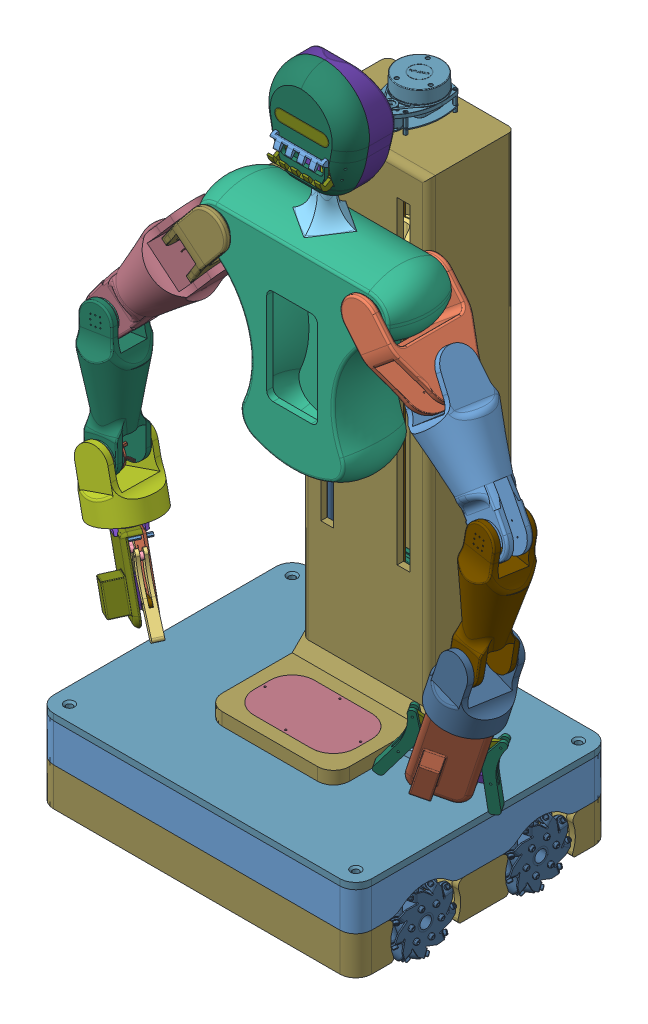
SolidWorks assembly total assembly of jaloul, configuration Défaut. Lengths in mm.
Overall size (783.33 1093.43 400).
399 component instances, 106 part files, 53 mates.
Components (placement in the parent):
- assembly bas robot jlayla-1: assembly bas robot jlayla [Défaut] at (49.7024 28.7761 8) size (508 175.73 400)
  - BASE ROBOT JALOUL-1: BASE ROBOT JALOUL [Défaut] at (-7.6983 -70.0077 500) size (500 80 400)
  - NEMA_235628-6.35_s.STEP-1: NEMA_235628-6.35_s.STEP [Défaut] at (-154.7901 -90.8073 611.8718) size (82 61.91 56.65)
    - Nema2356_top.STEP-1: Nema2356_top.STEP [Défaut] at (-25.5081 -82.6274 143.9932) size (12.4 56.42 56.42)
    - Nema2356_middle.STEP-1: Nema2356_middle.STEP [Défaut] at (-14.7081 17.769 14.044) size (32.8 56.4 56.4)
    - Nema2356_bottom.STEP-1: Nema2356_bottom.STEP [Défaut] at (18.0919 -112.7781 -165.2225) size (11 56.4 56.4)
    - Nema2356_axis.STEP-1: Nema2356_axis.STEP [Défaut] at (-52.9081 -12.2004 -20.8718) x (1 0 0) z (0 -0.367241 0.930126) size (78 6.35 6.35)
    - Nema2356_gultnis.STEP-1: Nema2356_gultnis.STEP [Défaut] at (-25.7081 -12.2004 -20.8718) x (1 0 0) z (0 0.415119 0.909767) size (3 11.6 11.6)
    - Nema2356_gultnis.STEP-2: Nema2356_gultnis.STEP [Défaut] at (22.0919 -12.2004 -20.8718) size (3 11.6 11.6)
    - Nema2356_screv.STEP-1: Nema2356_screv.STEP [Défaut] at (-13.1349 -28.2433 4.9528) size (54.01 5 5)
    - Nema2356_screv.STEP-2: Nema2356_screv.STEP [Défaut] at (-13.1349 3.8425 4.9528) size (54.01 5 5)
    - Nema2356_screv.STEP-3: Nema2356_screv.STEP [Défaut] at (-13.1349 -28.2433 -46.6964) size (54.01 5 5)
    - Nema2356_screv.STEP-4: Nema2356_screv.STEP [Défaut] at (-13.1349 3.8425 -46.6964) size (54.01 5 5)
    - Nema2356_contact.STEP-1: Nema2356_contact.STEP [Défaut] at (21.7519 15.9996 -20.8718) size (7.63 5.5 30.97)
  - support nema A 23 hee-1: support nema A 23 hee [Défaut] at (-180.2983 -103.0077 591) x (0 0 -1) z (-1 0 0) size (56 61 45)
  - Mecanum Wheel (dia 100)-1: Mecanum Wheel (dia 100) [Default] at (-192.6739 -101.7163 545.4553) x (0 -0.769085 0.639147) z (-1 0 0) size (104.21 104.22 58)
  - accouplement stpper with mecanum wheel-1: accouplement stpper with mecanum wheel [Défaut] at (-207.6983 -103.0077 591) x (0 -0.751439 0.659802) z (-1 0 0) size (18 18 35)
  - Mecanum Wheel (dia 100)-3: Mecanum Wheel (dia 100) [Default] at (177.2774 -146.933 583.0326) x (0 0.769085 -0.639147) z (1 0 0) size (104.21 104.22 58)
  - accouplement stpper with mecanum wheel-3: accouplement stpper with mecanum wheel [Défaut] at (192.3017 -103.0077 591) x (0 -0.751439 0.659802) z (1 0 0) size (18 18 35)
  - support nema A 23 hee-2: support nema A 23 hee [Défaut] at (164.9017 -103.0077 591) x (0 0 1) z (1 0 0) size (56 61 45)
  - Mecanum Wheel (dia 100)-4: Mecanum Wheel (dia 100) [Default] at (-192.6739 -146.933 416.9674) x (0 0.769085 0.639147) z (-1 0 0) size (104.21 104.22 58)
  - accouplement stpper with mecanum wheel-4: accouplement stpper with mecanum wheel [Défaut] at (-207.6983 -103.0077 409) x (0 -0.751439 -0.659802) z (-1 0 0) size (18 18 35)
  - support nema A 23 hee-3: support nema A 23 hee [Défaut] at (-180.2983 -103.0077 409) x (0 0 -1) z (-1 0 0) size (56 61 45)
  - support nema A 23 hee-4: support nema A 23 hee [Défaut] at (164.9017 -103.0077 409) x (0 0 1) z (1 0 0) size (56 61 45)
  - Mecanum Wheel (dia 100)-5: Mecanum Wheel (dia 100) [Default] at (177.2774 -102.9943 364.0959) x (0 0.769085 0.639147) z (1 0 0) size (104.21 104.22 58)
  - accouplement stpper with mecanum wheel-5: accouplement stpper with mecanum wheel [Défaut] at (192.3017 -103.0077 409) x (0 -0.751439 -0.659802) z (1 0 0) size (18 18 35)
  - NEMA_235628-6.35_s.STEP-2: NEMA_235628-6.35_s.STEP [Défaut] at (139.3936 -123.8795 578.7996) x (-1 0 0) z (0 -1 0) size (82 61.91 56.65)
    - Nema2356_top.STEP-1: Nema2356_top.STEP [Défaut] at (-25.5081 -82.6274 143.9932) size (12.4 56.42 56.42)
    - Nema2356_middle.STEP-1: Nema2356_middle.STEP [Défaut] at (-14.7081 17.769 14.044) size (32.8 56.4 56.4)
    - Nema2356_bottom.STEP-1: Nema2356_bottom.STEP [Défaut] at (18.0919 -112.7781 -165.2225) size (11 56.4 56.4)
    - Nema2356_axis.STEP-1: Nema2356_axis.STEP [Défaut] at (-52.9081 -12.2004 -20.8718) x (1 0 0) z (0 -0.367241 0.930126) size (78 6.35 6.35)
    - Nema2356_gultnis.STEP-1: Nema2356_gultnis.STEP [Défaut] at (-25.7081 -12.2004 -20.8718) x (1 0 0) z (0 0.415119 0.909767) size (3 11.6 11.6)
    - Nema2356_gultnis.STEP-2: Nema2356_gultnis.STEP [Défaut] at (22.0919 -12.2004 -20.8718) size (3 11.6 11.6)
    - Nema2356_screv.STEP-1: Nema2356_screv.STEP [Défaut] at (-13.1349 -28.2433 4.9528) size (54.01 5 5)
    - Nema2356_screv.STEP-2: Nema2356_screv.STEP [Défaut] at (-13.1349 3.8425 4.9528) size (54.01 5 5)
    - Nema2356_screv.STEP-3: Nema2356_screv.STEP [Défaut] at (-13.1349 -28.2433 -46.6964) size (54.01 5 5)
    - Nema2356_screv.STEP-4: Nema2356_screv.STEP [Défaut] at (-13.1349 3.8425 -46.6964) size (54.01 5 5)
    - Nema2356_contact.STEP-1: Nema2356_contact.STEP [Défaut] at (21.7519 15.9996 -20.8718) size (7.63 5.5 30.97)
  - NEMA_235628-6.35_s.STEP-3: NEMA_235628-6.35_s.STEP [Défaut] at (139.3936 -90.8073 388.1282) x (-1 0 0) z (0 0 -1) size (82 61.91 56.65)
    - Nema2356_top.STEP-1: Nema2356_top.STEP [Défaut] at (-25.5081 -82.6274 143.9932) size (12.4 56.42 56.42)
    - Nema2356_middle.STEP-1: Nema2356_middle.STEP [Défaut] at (-14.7081 17.769 14.044) size (32.8 56.4 56.4)
    - Nema2356_bottom.STEP-1: Nema2356_bottom.STEP [Défaut] at (18.0919 -112.7781 -165.2225) size (11 56.4 56.4)
    - Nema2356_axis.STEP-1: Nema2356_axis.STEP [Défaut] at (-52.9081 -12.2004 -20.8718) x (1 0 0) z (0 -0.367241 0.930126) size (78 6.35 6.35)
    - Nema2356_gultnis.STEP-1: Nema2356_gultnis.STEP [Défaut] at (-25.7081 -12.2004 -20.8718) x (1 0 0) z (0 0.415119 0.909767) size (3 11.6 11.6)
    - Nema2356_gultnis.STEP-2: Nema2356_gultnis.STEP [Défaut] at (22.0919 -12.2004 -20.8718) size (3 11.6 11.6)
    - Nema2356_screv.STEP-1: Nema2356_screv.STEP [Défaut] at (-13.1349 -28.2433 4.9528) size (54.01 5 5)
    - Nema2356_screv.STEP-2: Nema2356_screv.STEP [Défaut] at (-13.1349 3.8425 4.9528) size (54.01 5 5)
    - Nema2356_screv.STEP-3: Nema2356_screv.STEP [Défaut] at (-13.1349 -28.2433 -46.6964) size (54.01 5 5)
    - Nema2356_screv.STEP-4: Nema2356_screv.STEP [Défaut] at (-13.1349 3.8425 -46.6964) size (54.01 5 5)
    - Nema2356_contact.STEP-1: Nema2356_contact.STEP [Défaut] at (21.7519 15.9996 -20.8718) size (7.63 5.5 30.97)
  - NEMA_235628-6.35_s.STEP-4: NEMA_235628-6.35_s.STEP [Défaut] at (-154.7901 -90.8073 429.8718) size (82 61.91 56.65)
    - Nema2356_top.STEP-1: Nema2356_top.STEP [Défaut] at (-25.5081 -82.6274 143.9932) size (12.4 56.42 56.42)
    - Nema2356_middle.STEP-1: Nema2356_middle.STEP [Défaut] at (-14.7081 17.769 14.044) size (32.8 56.4 56.4)
    - Nema2356_bottom.STEP-1: Nema2356_bottom.STEP [Défaut] at (18.0919 -112.7781 -165.2225) size (11 56.4 56.4)
    - Nema2356_axis.STEP-1: Nema2356_axis.STEP [Défaut] at (-52.9081 -12.2004 -20.8718) x (1 0 0) z (0 -0.367241 0.930126) size (78 6.35 6.35)
    - Nema2356_gultnis.STEP-1: Nema2356_gultnis.STEP [Défaut] at (-25.7081 -12.2004 -20.8718) x (1 0 0) z (0 0.415119 0.909767) size (3 11.6 11.6)
    - Nema2356_gultnis.STEP-2: Nema2356_gultnis.STEP [Défaut] at (22.0919 -12.2004 -20.8718) size (3 11.6 11.6)
    - Nema2356_screv.STEP-1: Nema2356_screv.STEP [Défaut] at (-13.1349 -28.2433 4.9528) size (54.01 5 5)
    - Nema2356_screv.STEP-2: Nema2356_screv.STEP [Défaut] at (-13.1349 3.8425 4.9528) size (54.01 5 5)
    - Nema2356_screv.STEP-3: Nema2356_screv.STEP [Défaut] at (-13.1349 -28.2433 -46.6964) size (54.01 5 5)
    - Nema2356_screv.STEP-4: Nema2356_screv.STEP [Défaut] at (-13.1349 3.8425 -46.6964) size (54.01 5 5)
    - Nema2356_contact.STEP-1: Nema2356_contact.STEP [Défaut] at (21.7519 15.9996 -20.8718) size (7.63 5.5 30.97)
  - cache base joulayla-1: cache base joulayla [Défaut] at (-6.3132 -120.0077 499.8615) x (1 0 0) z (0 1 0) size (500 400 60)
  - profilé support base jlayla-1: profilé support base jlayla [Varsayılan] at (217.3017 -60.0077 675) x (1 0 0) z (0 1 0) size (25 25 50)
  - profilé support base jlayla-2: profilé support base jlayla [Varsayılan] at (-232.6983 -10.0077 675) x (-1 0 0) z (0 -1 0) size (25 25 50)
  - profilé support base jlayla-3: profilé support base jlayla [Varsayılan] at (217.3017 -10.0077 325) x (1 0 0) z (0 -1 0) size (25 25 50)
  - profilé support base jlayla-4: profilé support base jlayla [Varsayılan] at (-232.6983 -60.0077 325) x (-1 0 0) z (0 1 0) size (25 25 50)
  - profilé support base jlayla-5: profilé support base jlayla [Varsayılan] at (-7.6983 -60.0077 500) x (-1 0 0) z (0 1 0) size (25 25 50)
  - cache supérieur fixe jlayla-1: cache supérieur fixe jlayla [Défaut] at (-7.4213 -10.0077 499.0305) x (-1 0 0) z (0 1 0) size (500 400 10)
- assemblt jaloul main two-1: assemblt jaloul main two [Défaut] at (-8.2808 774.6085 403.5033) x (0.999385 -0.035073 0) z (0 0 1) size (752.19 900.92 286)
  - assembly head of jaloul-1: assembly head of jaloul [Défaut] at (50.4629 78.1935 73.0866) x (0.999385 0.035073 0) z (0 0 1) size (153.86 218.57 97.38)
    - head of jaloul-1: head of jaloul [Défaut] at (-2.8889 8.1989 56.9742) size (153.86 167.94 40.08)
    - RealSense_D435-1: RealSense_D435 [Default] at (-2 5.7058 43.2445) size (90.75 24.75 24.23)
    - ras jaloul men teli-1: ras jaloul men teli [Défaut] at (-4.3071 -4.0651 25.143) size (140.75 169.26 46.26)
    - raspberry-pi-5-sbc-simple.step-1: raspberry-pi-5-sbc-simple.step [Défaut] at (-2.8895 30.0633 18.143) size (90.56 58 19.2)
      - CSI_DSI-1.step-1: CSI_DSI-1.step [Défaut] at (-70.5 -36 11.75) size (3 15.5 4.1)
        - CSI_DSI_connector.step-1: CSI_DSI_connector.step [Défaut] at origin size (3 15.5 4.1)
      - CSI_DSI-2.step-1: CSI_DSI-2.step [Défaut] at (-70.5 -36 11.75) size (3 15.5 4.1)
        - CSI_DSI_connector.step-1: CSI_DSI_connector.step [Défaut] at (6.2 0 0) size (3 15.5 4.1)
      - pcba-components.step-1: pcba-components.step [Défaut] at (-70.5 -36 11.75) size (64.89 40.96 3.37)
        - pcba-components Geometry.step-1: pcba-components Geometry.step [Défaut] at origin size (62.02 39.27 3.37)
        - chips.step-1: chips.step [Défaut] at origin size (13.6 15 1)
      - poe.step-1: poe.step [Défaut] at (-70.5 -36 11.75) size (5.08 5.08 8.29)
        - poe Geometry.step-1: poe Geometry.step [Défaut] at origin size (5.08 5.08 1)
        - poe-pins.step-1: poe-pins.step [Défaut] at origin size (3.44 3.44 7.29)
      - usb-2-bank.step-1: usb-2-bank.step [Défaut] at (-0.7443 20 0.8) x (1 0 0) z (0 -1 0) size (17.07 15.5 13.76)
        - usb-2-bank Geometry.step-1: usb-2-bank Geometry.step [Défaut] at origin size (16.67 15.5 13.76)
        - usb2-port.step-1: usb2-port.step [Défaut] at origin size (4.42 5.12 12.5)
        - usb2-port.step-2: usb2-port.step [Défaut] at (0 -8.5 0) size (4.42 5.12 12.5)
      - usb-3-bank.step-1: usb-3-bank.step [Défaut] at (-0.5443 2.1 0.8) x (1 0 0) z (0 -1 0) size (17.07 15.5 13.76)
        - usb-3-bank Geometry.step-1: usb-3-bank Geometry.step [Défaut] at origin size (16.67 15.5 13.76)
        - usb3-port.step-1: usb3-port.step [Défaut] at origin size (4.42 5.12 12.5)
        - usb3-port.step-2: usb3-port.step [Défaut] at (0 -8.5 0) size (4.42 5.12 12.5)
      - connector.step-1: connector.step [Défaut] at (-70.5 -36 11.75) size (3 6 3.5)
      - ethernet.step-1: ethernet.step [Défaut] at (0 -35.55 0.8) x (1 0 0) z (0 -1 0) size (23.65 17.25 16)
      - gpio.step-1: gpio.step [Défaut] at (-70.53 -36.28 11.75) size (50.5 5 8.29)
      - hdmi-micro.step-1: hdmi-micro.step [Défaut] at (-0.3 0 0.8) x (1 0 0) z (0 -1 0) size (6.5 2.9 7.7)
      - hdmi-micro.step-2: hdmi-micro.step [Défaut] at (-13.8 0 0.8) x (1 0 0) z (0 -1 0) size (6.5 2.9 7.7)
      - IR.step-1: IR.step [Défaut] at (-70.5 -36 11.75) size (1.73 3.15 3.26)
      - mounting-holes.step-1: mounting-holes.step [Défaut] at (-70.5 -36 11.75) size (64 54.91 0.02)
      - pcb.step-1: pcb.step [Défaut] at (-70.5 -36 11.75) size (85 56 1.6)
      - pcie.step-1: pcie.step [Défaut] at (-70.5 -36 11.75) size (3 10.5 4.1)
      - pmic.step-1: pmic.step [Défaut] at (-70.5 -36 11.75) size (6 6 0.5)
      - pwr-connector.step-1: pwr-connector.step [Défaut] at (-70.5 -36 11.75) size (4 3 4.4)
      - rp1.step-1: rp1.step [Défaut] at (-70.5 -36 11.75) size (12 12 0.5)
      - sd-card.step-1: sd-card.step [Défaut] at (-70.5 -36 11.75) size (1.75 11.01 0.01) (hidden)
      - switch.step-1: switch.step [Défaut] at (-70.5 -36 11.75) size (3 4.75 1.77)
      - uart.step-1: uart.step [Défaut] at (-70.5 -36 11.75) size (5.25 3.25 4.4)
      - usb-c.step-1: usb-c.step [Défaut] at (-70.5 -36 11.75) size (9 7.5 3.2)
    - support head-1: support head [Défaut] at (-2.8895 -82.9367 30.143) x (0.544466 0 -0.838783) z (0 -1 0) size (62.95 62.95 55.38)
    - M90S_ali.step-1: M90S_ali.step [Défaut] at (23.3 -47.0367 54.243) x (0 -1 0) z (1 0 0) size (32.3 12.4 32.5)
      - axe.step-1: axe.step [Défaut] at origin size (4.9 4.9 14.2)
      - base001.step-1: base001.step [Défaut] at origin size (32.3 12.2 28.5)
      - etiquette.step-1: etiquette.step [Défaut] at origin size (20 0.2 10)
      - Tube.step-1: Tube.step [Défaut] at (5.4 0 -13.3) x (0 0 -1) z (1 0 0) size (1.2 1.2 3)
      - Cylindre.step-1: Cylindre.step [Défaut] at (5.4 0 -13.3) x (0 0 -1) z (1 0 0) size (0.4 0.4 4)
      - Tube001.step-1: Tube001.step [Défaut] at (5.4 -1.2 -13.3) x (0 0 -1) z (1 0 0) size (1.2 1.2 3)
      - Tube002.step-1: Tube002.step [Défaut] at (5.4 1.2 -13.3) x (0 0 -1) z (1 0 0) size (1.2 1.2 3)
      - etiquette001.step-1: etiquette001.step [Défaut] at (-10.8 0 0) x (-1 0 0) z (0 0 1) size (20 0.2 10)
      - Cylindre001.step-1: Cylindre001.step [Défaut] at (5.4 1.2 -13.3) x (0 0 -1) z (1 0 0) size (0.4 0.4 4)
      - Cylindre002.step-1: Cylindre002.step [Défaut] at (5.4 -1.2 -13.3) x (0 0 -1) z (1 0 0) size (0.4 0.4 4)
    - dents du jaloul-1: dents du jaloul [Défaut] at (-1.85 -55.3304 58.7391) x (-1 0 0) z (0 0.870081 0.492909) size (83 33.18 25.45)
    - MG90S_arm01.step-1: MG90S_arm01.step [Défaut] at (39.3 -47.0367 54.243) x (-1 0 0) z (0 0.870081 0.492909) size (4.8 21.4 6.8)
    - dent jaloul partie supérieur-1: dent jaloul partie supérieur [Défaut] at (-1.85 5.574 3.1017) size (83 33.18 25.45)
    - Symétriedents du jaloul-4: Symétriedents du jaloul [Défaut] at (-1.85 -21.043 58.7391) x (-1 0 0) z (0 0.870081 -0.492909) size (83 32.99 25.26)
  - 4015 Motor.STEP-1: 4015 Motor.STEP [Défaut] at (-65.9697 -107.9474 135.4967) x (-0.675127 -0.737702 0) z (-0.737702 0.675127 0) size (63.54 36.6 63.54)
    - 4015定子.STEP-1: 4015定子.STEP [Défaut] at origin size (45.94 27.09 45.92)
    - MISUMI_C-E6800ZZ.STEP-1: MISUMI_C-E6800ZZ.STEP [Défaut] at (0 21.6 0) x (0 -1 0) z (-0.009932 0 0.999951) size (5 19 19)
    - MISUMI_C-E6800ZZ.STEP-2: MISUMI_C-E6800ZZ.STEP [Défaut] at (0 8 0) x (0 -1 0) z (-0.587995 0 0.808864) size (5 19 19)
    - 转子铝盖.STEP-1: 转子铝盖.STEP [Défaut] at (0 24 0) x (-0.665718 0 -0.746203) z (-0.746203 0 0.665718) size (45 23.5 45)
    - 磁钢片.STEP-1: 磁钢片.STEP [Défaut] at (5.7872 12.75 -20.8182) x (0.963466 0 0.267832) z (-0.267832 0 0.963466) size (4 16.5 1.3)
    - 中间不锈钢圈.STEP-1: 中间不锈钢圈.STEP [Défaut] at (0 4.5 0) x (0.999998 0 0.002002) z (0 1 0) size (45 45 16.5)
    - 磁钢片.STEP-2: 磁钢片.STEP [Défaut] at (-0.3124 12.75 -21.6054) x (0.999895 0 -0.014457) z (0.014457 0 0.999895) size (4 16.5 1.3)
    - 磁钢片.STEP-3: 磁钢片.STEP [Défaut] at (-6.3867 12.75 -20.6422) x (0.95532 0 -0.295574) z (0.295574 0 0.95532) size (4 16.5 1.3)
    - 磁钢片.STEP-4: 磁钢片.STEP [Défaut] at (-11.9435 12.75 -18.0067) x (0.83335 0 -0.552746) z (0.552746 0 0.83335) size (4 16.5 1.3)
    - 磁钢片.STEP-5: 磁钢片.STEP [Défaut] at (-16.5328 12.75 -13.9124) x (0.643867 0 -0.765138) z (0.765138 0 0.643867) size (4 16.5 1.3)
    - 磁钢片.STEP-6: 磁钢片.STEP [Défaut] at (-19.7827 12.75 -8.6911) x (0.402221 0 -0.915542) z (0.915542 0 0.402221) size (4 16.5 1.3)
    - 磁钢片.STEP-7: 磁钢片.STEP [Défaut] at (-21.4299 12.75 -2.7656) x (0.12799 0 -0.991775) z (0.991775 0 0.12799) size (4 16.5 1.3)
    - 磁钢片.STEP-8: 磁钢片.STEP [Défaut] at (-21.341 12.75 3.384) x (-0.15661 0 -0.987661) z (0.987661 0 -0.15661) size (4 16.5 1.3)
    - 磁钢片.STEP-9: 磁钢片.STEP [Défaut] at (-19.5232 12.75 9.2593) x (-0.428522 0 -0.903531) z (0.903531 0 -0.428522) size (4 16.5 1.3)
    - 磁钢片.STEP-10: 磁钢片.STEP [Défaut] at (-16.1237 12.75 14.3846) x (-0.665718 0 -0.746203) z (0.746203 0 -0.665718) size (4 16.5 1.3)
    - 磁钢片.STEP-11: 磁钢片.STEP [Défaut] at (-11.418 12.75 18.3445) x (-0.848982 0 -0.528423) z (0.528423 0 -0.848982) size (4 16.5 1.3)
    - 磁钢片.STEP-12: 磁钢片.STEP [Défaut] at (-5.7872 12.75 20.8182) x (-0.963466 0 -0.267832) z (0.267832 0 -0.963466) size (4 16.5 1.3)
    - 磁钢片.STEP-13: 磁钢片.STEP [Défaut] at (0.3124 12.75 21.6054) x (-0.999895 0 0.014457) z (-0.014457 0 -0.999895) size (4 16.5 1.3)
    - 磁钢片.STEP-14: 磁钢片.STEP [Défaut] at (6.3867 12.75 20.6422) x (-0.95532 0 0.295574) z (-0.295574 0 -0.95532) size (4 16.5 1.3)
    - 磁钢片.STEP-15: 磁钢片.STEP [Défaut] at (11.9435 12.75 18.0067) x (-0.83335 0 0.552746) z (-0.552746 0 -0.83335) size (4 16.5 1.3)
    - 磁钢片.STEP-16: 磁钢片.STEP [Défaut] at (16.5328 12.75 13.9124) x (-0.643867 0 0.765138) z (-0.765138 0 -0.643867) size (4 16.5 1.3)
    - 磁钢片.STEP-17: 磁钢片.STEP [Défaut] at (19.7827 12.75 8.6911) x (-0.402221 0 0.915542) z (-0.915542 0 -0.402221) size (4 16.5 1.3)
    - 磁钢片.STEP-18: 磁钢片.STEP [Défaut] at (21.4299 12.75 2.7656) x (-0.12799 0 0.991775) z (-0.991775 0 -0.12799) size (4 16.5 1.3)
    - 磁钢片.STEP-19: 磁钢片.STEP [Défaut] at (21.341 12.75 -3.384) x (0.15661 0 0.987661) z (-0.987661 0 0.15661) size (4 16.5 1.3)
    - 磁钢片.STEP-20: 磁钢片.STEP [Défaut] at (19.5232 12.75 -9.2593) x (0.428522 0 0.903531) z (-0.903531 0 0.428522) size (4 16.5 1.3)
    - 磁钢片.STEP-21: 磁钢片.STEP [Défaut] at (16.1237 12.75 -14.3846) x (0.665718 0 0.746203) z (-0.746203 0 0.665718) size (4 16.5 1.3)
    - 磁钢片.STEP-22: 磁钢片.STEP [Défaut] at (11.418 12.75 -18.3445) x (0.848982 0 0.528423) z (-0.528423 0 0.848982) size (4 16.5 1.3)
    - 径向磁环.STEP-1: 径向磁环.STEP [Défaut] at (0 0.5 0) x (0.972164 0 0.234302) z (0 -1 0) size (10 10 2.5)
    - 径向磁环固定环.STEP-1: 径向磁环固定环.STEP [Défaut] at (0 -2 0) x (0.933781 0 0.357846) z (0 1 0) size (11.2 12.93 5)
    - 铜柱M2.5x4+4.STEP-1: 铜柱M2.5x4+4.STEP [Défaut] at (14 -4 0) size (5 8 5.77)
    - 铜柱M2.5x4+4.STEP-2: 铜柱M2.5x4+4.STEP [Défaut] at (0 -4 -14) x (0.982082 0 -0.188455) z (0.188455 0 0.982082) size (5 8 5.77)
    - 铜柱M2.5x4+4.STEP-3: 铜柱M2.5x4+4.STEP [Défaut] at (0 -4 14) x (0.918365 0 -0.395734) z (0.395734 0 0.918365) size (5 8 5.77)
    - 铜柱M2.5x4+4.STEP-4: 铜柱M2.5x4+4.STEP [Défaut] at (-14 -4 0) x (0.8 0 -0.6) z (0.6 0 0.8) size (5 8 5.77)
    - AS5600磁编码器-圆.STEP-1: AS5600磁编码器-圆.STEP [Défaut] at (-0.3592 -5.6 0) x (0.707107 0 -0.707107) z (0 1 0) size (31.97 31.97 7.67)
    - 铜柱M2.5x7+4.STEP-1: 铜柱M2.5x7+4.STEP [Défaut] at (0 -12.6 -14) x (0.898383 0 -0.439214) z (0.439214 0 0.898383) size (5 11 5.77)
    - 铜柱M2.5x7+4.STEP-2: 铜柱M2.5x7+4.STEP [Défaut] at (-14 -12.6 0) x (0.799513 0 -0.600648) z (0.600648 0 0.799513) size (5 11 5.77)
    - 铜柱M2.5x7+4.STEP-3: 铜柱M2.5x7+4.STEP [Défaut] at (14 -12.6 0) x (0.651231 0 -0.758879) z (0.758879 0 0.651231) size (5 11 5.77)
    - 铜柱M2.5x7+4.STEP-4: 铜柱M2.5x7+4.STEP [Défaut] at (0 -12.6 14) x (0.455178 0 -0.890401) z (0.890401 0 0.455178) size (5 11 5.77)
  - link 1 JALOUL-1: link 1 JALOUL [Défaut] at (-74.3576 -118.8426 159.4967) x (0.61003 0.792378 0) z (0 0 1) size (167.5 60.6 125)
  - 4015 Motor.STEP-2: 4015 Motor.STEP [Défaut] at (-134.1638 -178.494 106.9967) x (0.604333 0.784978 0.136349) z (-0.083177 -0.10804 0.990661) size (63.54 36.6 63.54)
    - 4015定子.STEP-1: 4015定子.STEP [Défaut] at origin size (45.94 27.09 45.92)
    - MISUMI_C-E6800ZZ.STEP-1: MISUMI_C-E6800ZZ.STEP [Défaut] at (0 21.6 0) x (0 -1 0) z (-0.009932 0 0.999951) size (5 19 19)
    - MISUMI_C-E6800ZZ.STEP-2: MISUMI_C-E6800ZZ.STEP [Défaut] at (0 8 0) x (0 -1 0) z (-0.587995 0 0.808864) size (5 19 19)
    - 转子铝盖.STEP-1: 转子铝盖.STEP [Défaut] at (0 24 0) x (-0.665718 0 -0.746203) z (-0.746203 0 0.665718) size (45 23.5 45)
    - 磁钢片.STEP-1: 磁钢片.STEP [Défaut] at (5.7872 12.75 -20.8182) x (0.963466 0 0.267832) z (-0.267832 0 0.963466) size (4 16.5 1.3)
    - 中间不锈钢圈.STEP-1: 中间不锈钢圈.STEP [Défaut] at (0 4.5 0) x (0.999998 0 0.002002) z (0 1 0) size (45 45 16.5)
    - 磁钢片.STEP-2: 磁钢片.STEP [Défaut] at (-0.3124 12.75 -21.6054) x (0.999895 0 -0.014457) z (0.014457 0 0.999895) size (4 16.5 1.3)
    - 磁钢片.STEP-3: 磁钢片.STEP [Défaut] at (-6.3867 12.75 -20.6422) x (0.95532 0 -0.295574) z (0.295574 0 0.95532) size (4 16.5 1.3)
    - 磁钢片.STEP-4: 磁钢片.STEP [Défaut] at (-11.9435 12.75 -18.0067) x (0.83335 0 -0.552746) z (0.552746 0 0.83335) size (4 16.5 1.3)
    - 磁钢片.STEP-5: 磁钢片.STEP [Défaut] at (-16.5328 12.75 -13.9124) x (0.643867 0 -0.765138) z (0.765138 0 0.643867) size (4 16.5 1.3)
    - 磁钢片.STEP-6: 磁钢片.STEP [Défaut] at (-19.7827 12.75 -8.6911) x (0.402221 0 -0.915542) z (0.915542 0 0.402221) size (4 16.5 1.3)
    - 磁钢片.STEP-7: 磁钢片.STEP [Défaut] at (-21.4299 12.75 -2.7656) x (0.12799 0 -0.991775) z (0.991775 0 0.12799) size (4 16.5 1.3)
    - 磁钢片.STEP-8: 磁钢片.STEP [Défaut] at (-21.341 12.75 3.384) x (-0.15661 0 -0.987661) z (0.987661 0 -0.15661) size (4 16.5 1.3)
    - 磁钢片.STEP-9: 磁钢片.STEP [Défaut] at (-19.5232 12.75 9.2593) x (-0.428522 0 -0.903531) z (0.903531 0 -0.428522) size (4 16.5 1.3)
    - 磁钢片.STEP-10: 磁钢片.STEP [Défaut] at (-16.1237 12.75 14.3846) x (-0.665718 0 -0.746203) z (0.746203 0 -0.665718) size (4 16.5 1.3)
    - 磁钢片.STEP-11: 磁钢片.STEP [Défaut] at (-11.418 12.75 18.3445) x (-0.848982 0 -0.528423) z (0.528423 0 -0.848982) size (4 16.5 1.3)
    - 磁钢片.STEP-12: 磁钢片.STEP [Défaut] at (-5.7872 12.75 20.8182) x (-0.963466 0 -0.267832) z (0.267832 0 -0.963466) size (4 16.5 1.3)
    - 磁钢片.STEP-13: 磁钢片.STEP [Défaut] at (0.3124 12.75 21.6054) x (-0.999895 0 0.014457) z (-0.014457 0 -0.999895) size (4 16.5 1.3)
    - 磁钢片.STEP-14: 磁钢片.STEP [Défaut] at (6.3867 12.75 20.6422) x (-0.95532 0 0.295574) z (-0.295574 0 -0.95532) size (4 16.5 1.3)
    - 磁钢片.STEP-15: 磁钢片.STEP [Défaut] at (11.9435 12.75 18.0067) x (-0.83335 0 0.552746) z (-0.552746 0 -0.83335) size (4 16.5 1.3)
    - 磁钢片.STEP-16: 磁钢片.STEP [Défaut] at (16.5328 12.75 13.9124) x (-0.643867 0 0.765138) z (-0.765138 0 -0.643867) size (4 16.5 1.3)
    - 磁钢片.STEP-17: 磁钢片.STEP [Défaut] at (19.7827 12.75 8.6911) x (-0.402221 0 0.915542) z (-0.915542 0 -0.402221) size (4 16.5 1.3)
    - 磁钢片.STEP-18: 磁钢片.STEP [Défaut] at (21.4299 12.75 2.7656) x (-0.12799 0 0.991775) z (-0.991775 0 -0.12799) size (4 16.5 1.3)
    - 磁钢片.STEP-19: 磁钢片.STEP [Défaut] at (21.341 12.75 -3.384) x (0.15661 0 0.987661) z (-0.987661 0 0.15661) size (4 16.5 1.3)
    - 磁钢片.STEP-20: 磁钢片.STEP [Défaut] at (19.5232 12.75 -9.2593) x (0.428522 0 0.903531) z (-0.903531 0 0.428522) size (4 16.5 1.3)
    - 磁钢片.STEP-21: 磁钢片.STEP [Défaut] at (16.1237 12.75 -14.3846) x (0.665718 0 0.746203) z (-0.746203 0 0.665718) size (4 16.5 1.3)
    - 磁钢片.STEP-22: 磁钢片.STEP [Défaut] at (11.418 12.75 -18.3445) x (0.848982 0 0.528423) z (-0.528423 0 0.848982) size (4 16.5 1.3)
    - 径向磁环.STEP-1: 径向磁环.STEP [Défaut] at (0 0.5 0) x (0.972164 0 0.234302) z (0 -1 0) size (10 10 2.5)
    - 径向磁环固定环.STEP-1: 径向磁环固定环.STEP [Défaut] at (0 -2 0) x (0.933781 0 0.357846) z (0 1 0) size (11.2 12.93 5)
    - 铜柱M2.5x4+4.STEP-1: 铜柱M2.5x4+4.STEP [Défaut] at (14 -4 0) size (5 8 5.77)
    - 铜柱M2.5x4+4.STEP-2: 铜柱M2.5x4+4.STEP [Défaut] at (0 -4 -14) x (0.982082 0 -0.188455) z (0.188455 0 0.982082) size (5 8 5.77)
    - 铜柱M2.5x4+4.STEP-3: 铜柱M2.5x4+4.STEP [Défaut] at (0 -4 14) x (0.918365 0 -0.395734) z (0.395734 0 0.918365) size (5 8 5.77)
    - 铜柱M2.5x4+4.STEP-4: 铜柱M2.5x4+4.STEP [Défaut] at (-14 -4 0) x (0.8 0 -0.6) z (0.6 0 0.8) size (5 8 5.77)
    - AS5600磁编码器-圆.STEP-1: AS5600磁编码器-圆.STEP [Défaut] at (-0.3592 -5.6 0) x (0.707107 0 -0.707107) z (0 1 0) size (31.97 31.97 7.67)
    - 铜柱M2.5x7+4.STEP-1: 铜柱M2.5x7+4.STEP [Défaut] at (0 -12.6 -14) x (0.898383 0 -0.439214) z (0.439214 0 0.898383) size (5 11 5.77)
    - 铜柱M2.5x7+4.STEP-2: 铜柱M2.5x7+4.STEP [Défaut] at (-14 -12.6 0) x (0.799513 0 -0.600648) z (0.600648 0 0.799513) size (5 11 5.77)
    - 铜柱M2.5x7+4.STEP-3: 铜柱M2.5x7+4.STEP [Défaut] at (14 -12.6 0) x (0.651231 0 -0.758879) z (0.758879 0 0.651231) size (5 11 5.77)
    - 铜柱M2.5x7+4.STEP-4: 铜柱M2.5x7+4.STEP [Défaut] at (0 -12.6 14) x (0.455178 0 -0.890401) z (0.890401 0 0.455178) size (5 11 5.77)
  - link 2 JALOUL-1: link 2 JALOUL [Défaut] at (-194.9505 -201.7159 82.9556) x (0.606326 0.787567 -0.110033) z (0.067124 0.087188 0.993928) size (247.23 121.75 118.52)
  - 4015 Motor.STEP-3: 4015 Motor.STEP [Défaut] at (-242.3982 -333.0153 128.8669) x (-0.985892 -0.147294 0.079502) z (-0.153331 0.985242 -0.076071) size (63.54 36.6 63.54)
    - 4015定子.STEP-1: 4015定子.STEP [Défaut] at origin size (45.94 27.09 45.92)
    - MISUMI_C-E6800ZZ.STEP-1: MISUMI_C-E6800ZZ.STEP [Défaut] at (0 21.6 0) x (0 -1 0) z (-0.009932 0 0.999951) size (5 19 19)
    - MISUMI_C-E6800ZZ.STEP-2: MISUMI_C-E6800ZZ.STEP [Défaut] at (0 8 0) x (0 -1 0) z (-0.587995 0 0.808864) size (5 19 19)
    - 转子铝盖.STEP-1: 转子铝盖.STEP [Défaut] at (0 24 0) x (-0.665718 0 -0.746203) z (-0.746203 0 0.665718) size (45 23.5 45)
    - 磁钢片.STEP-1: 磁钢片.STEP [Défaut] at (5.7872 12.75 -20.8182) x (0.963466 0 0.267832) z (-0.267832 0 0.963466) size (4 16.5 1.3)
    - 中间不锈钢圈.STEP-1: 中间不锈钢圈.STEP [Défaut] at (0 4.5 0) x (0.999998 0 0.002002) z (0 1 0) size (45 45 16.5)
    - 磁钢片.STEP-2: 磁钢片.STEP [Défaut] at (-0.3124 12.75 -21.6054) x (0.999895 0 -0.014457) z (0.014457 0 0.999895) size (4 16.5 1.3)
    - 磁钢片.STEP-3: 磁钢片.STEP [Défaut] at (-6.3867 12.75 -20.6422) x (0.95532 0 -0.295574) z (0.295574 0 0.95532) size (4 16.5 1.3)
    - 磁钢片.STEP-4: 磁钢片.STEP [Défaut] at (-11.9435 12.75 -18.0067) x (0.83335 0 -0.552746) z (0.552746 0 0.83335) size (4 16.5 1.3)
    - 磁钢片.STEP-5: 磁钢片.STEP [Défaut] at (-16.5328 12.75 -13.9124) x (0.643867 0 -0.765138) z (0.765138 0 0.643867) size (4 16.5 1.3)
    - 磁钢片.STEP-6: 磁钢片.STEP [Défaut] at (-19.7827 12.75 -8.6911) x (0.402221 0 -0.915542) z (0.915542 0 0.402221) size (4 16.5 1.3)
    - 磁钢片.STEP-7: 磁钢片.STEP [Défaut] at (-21.4299 12.75 -2.7656) x (0.12799 0 -0.991775) z (0.991775 0 0.12799) size (4 16.5 1.3)
    - 磁钢片.STEP-8: 磁钢片.STEP [Défaut] at (-21.341 12.75 3.384) x (-0.15661 0 -0.987661) z (0.987661 0 -0.15661) size (4 16.5 1.3)
    - 磁钢片.STEP-9: 磁钢片.STEP [Défaut] at (-19.5232 12.75 9.2593) x (-0.428522 0 -0.903531) z (0.903531 0 -0.428522) size (4 16.5 1.3)
    - 磁钢片.STEP-10: 磁钢片.STEP [Défaut] at (-16.1237 12.75 14.3846) x (-0.665718 0 -0.746203) z (0.746203 0 -0.665718) size (4 16.5 1.3)
    - 磁钢片.STEP-11: 磁钢片.STEP [Défaut] at (-11.418 12.75 18.3445) x (-0.848982 0 -0.528423) z (0.528423 0 -0.848982) size (4 16.5 1.3)
    - 磁钢片.STEP-12: 磁钢片.STEP [Défaut] at (-5.7872 12.75 20.8182) x (-0.963466 0 -0.267832) z (0.267832 0 -0.963466) size (4 16.5 1.3)
    - 磁钢片.STEP-13: 磁钢片.STEP [Défaut] at (0.3124 12.75 21.6054) x (-0.999895 0 0.014457) z (-0.014457 0 -0.999895) size (4 16.5 1.3)
    - 磁钢片.STEP-14: 磁钢片.STEP [Défaut] at (6.3867 12.75 20.6422) x (-0.95532 0 0.295574) z (-0.295574 0 -0.95532) size (4 16.5 1.3)
    - 磁钢片.STEP-15: 磁钢片.STEP [Défaut] at (11.9435 12.75 18.0067) x (-0.83335 0 0.552746) z (-0.552746 0 -0.83335) size (4 16.5 1.3)
    - 磁钢片.STEP-16: 磁钢片.STEP [Défaut] at (16.5328 12.75 13.9124) x (-0.643867 0 0.765138) z (-0.765138 0 -0.643867) size (4 16.5 1.3)
    - 磁钢片.STEP-17: 磁钢片.STEP [Défaut] at (19.7827 12.75 8.6911) x (-0.402221 0 0.915542) z (-0.915542 0 -0.402221) size (4 16.5 1.3)
    - 磁钢片.STEP-18: 磁钢片.STEP [Défaut] at (21.4299 12.75 2.7656) x (-0.12799 0 0.991775) z (-0.991775 0 -0.12799) size (4 16.5 1.3)
    - 磁钢片.STEP-19: 磁钢片.STEP [Défaut] at (21.341 12.75 -3.384) x (0.15661 0 0.987661) z (-0.987661 0 0.15661) size (4 16.5 1.3)
    - 磁钢片.STEP-20: 磁钢片.STEP [Défaut] at (19.5232 12.75 -9.2593) x (0.428522 0 0.903531) z (-0.903531 0 0.428522) size (4 16.5 1.3)
    - 磁钢片.STEP-21: 磁钢片.STEP [Défaut] at (16.1237 12.75 -14.3846) x (0.665718 0 0.746203) z (-0.746203 0 0.665718) size (4 16.5 1.3)
    - 磁钢片.STEP-22: 磁钢片.STEP [Défaut] at (11.418 12.75 -18.3445) x (0.848982 0 0.528423) z (-0.528423 0 0.848982) size (4 16.5 1.3)
    - 径向磁环.STEP-1: 径向磁环.STEP [Défaut] at (0 0.5 0) x (0.972164 0 0.234302) z (0 -1 0) size (10 10 2.5)
    - 径向磁环固定环.STEP-1: 径向磁环固定环.STEP [Défaut] at (0 -2 0) x (0.933781 0 0.357846) z (0 1 0) size (11.2 12.93 5)
    - 铜柱M2.5x4+4.STEP-1: 铜柱M2.5x4+4.STEP [Défaut] at (14 -4 0) size (5 8 5.77)
    - 铜柱M2.5x4+4.STEP-2: 铜柱M2.5x4+4.STEP [Défaut] at (0 -4 -14) x (0.982082 0 -0.188455) z (0.188455 0 0.982082) size (5 8 5.77)
    - 铜柱M2.5x4+4.STEP-3: 铜柱M2.5x4+4.STEP [Défaut] at (0 -4 14) x (0.918365 0 -0.395734) z (0.395734 0 0.918365) size (5 8 5.77)
    - 铜柱M2.5x4+4.STEP-4: 铜柱M2.5x4+4.STEP [Défaut] at (-14 -4 0) x (0.8 0 -0.6) z (0.6 0 0.8) size (5 8 5.77)
    - AS5600磁编码器-圆.STEP-1: AS5600磁编码器-圆.STEP [Défaut] at (-0.3592 -5.6 0) x (0.707107 0 -0.707107) z (0 1 0) size (31.97 31.97 7.67)
    - 铜柱M2.5x7+4.STEP-1: 铜柱M2.5x7+4.STEP [Défaut] at (0 -12.6 -14) x (0.898383 0 -0.439214) z (0.439214 0 0.898383) size (5 11 5.77)
    - 铜柱M2.5x7+4.STEP-2: 铜柱M2.5x7+4.STEP [Défaut] at (-14 -12.6 0) x (0.799513 0 -0.600648) z (0.600648 0 0.799513) size (5 11 5.77)
    - 铜柱M2.5x7+4.STEP-3: 铜柱M2.5x7+4.STEP [Défaut] at (14 -12.6 0) x (0.651231 0 -0.758879) z (0.758879 0 0.651231) size (5 11 5.77)
    - 铜柱M2.5x7+4.STEP-4: 铜柱M2.5x7+4.STEP [Défaut] at (0 -12.6 14) x (0.455178 0 -0.890401) z (0.890401 0 0.455178) size (5 11 5.77)
  - ISO 15 RBB - 105 - 8,SI,NC,8_68-1: ISO 15 RBB - 105 - 8,SI,NC,8_68 [ISO 15 RBB - 105 - 8,SI,NC,8_68] at (-316.6056 -16.061 376.3383) x (0.875338 0.056415 0.480209) z (0.163001 -0.969462 -0.18323) size (5 14 14) (hidden)
  - ISO 15 RBB - 105 - 8,SI,NC,8_68-2: ISO 15 RBB - 105 - 8,SI,NC,8_68 [ISO 15 RBB - 105 - 8,SI,NC,8_68] at (-108.995 -208.9135 106.9967) x (0.792378 -0.61003 0) z (0 0 1) size (5 14 14)
  - LINK 3 JALOUL-1: LINK 3 JALOUL [Défaut] at (-257.529 -387.5668 168.8818) x (-0.13288 0.988082 -0.077701) z (0.988857 0.126858 -0.077909) size (224.5 90.56 90.03)
  - 4015 Motor.STEP-5: 4015 Motor.STEP [Défaut] at (-218.4729 -505.0577 152.4039) x (-0.746862 0.664932 -0.00789) z (0.661582 0.741798 -0.10975) size (63.54 36.6 63.54)
    - 4015定子.STEP-1: 4015定子.STEP [Défaut] at origin size (45.94 27.09 45.92)
    - MISUMI_C-E6800ZZ.STEP-1: MISUMI_C-E6800ZZ.STEP [Défaut] at (0 21.6 0) x (0 -1 0) z (-0.009932 0 0.999951) size (5 19 19)
    - MISUMI_C-E6800ZZ.STEP-2: MISUMI_C-E6800ZZ.STEP [Défaut] at (0 8 0) x (0 -1 0) z (-0.587995 0 0.808864) size (5 19 19)
    - 转子铝盖.STEP-1: 转子铝盖.STEP [Défaut] at (0 24 0) x (-0.665718 0 -0.746203) z (-0.746203 0 0.665718) size (45 23.5 45)
    - 磁钢片.STEP-1: 磁钢片.STEP [Défaut] at (5.7872 12.75 -20.8182) x (0.963466 0 0.267832) z (-0.267832 0 0.963466) size (4 16.5 1.3)
    - 中间不锈钢圈.STEP-1: 中间不锈钢圈.STEP [Défaut] at (0 4.5 0) x (0.999998 0 0.002002) z (0 1 0) size (45 45 16.5)
    - 磁钢片.STEP-2: 磁钢片.STEP [Défaut] at (-0.3124 12.75 -21.6054) x (0.999895 0 -0.014457) z (0.014457 0 0.999895) size (4 16.5 1.3)
    - 磁钢片.STEP-3: 磁钢片.STEP [Défaut] at (-6.3867 12.75 -20.6422) x (0.95532 0 -0.295574) z (0.295574 0 0.95532) size (4 16.5 1.3)
    - 磁钢片.STEP-4: 磁钢片.STEP [Défaut] at (-11.9435 12.75 -18.0067) x (0.83335 0 -0.552746) z (0.552746 0 0.83335) size (4 16.5 1.3)
    - 磁钢片.STEP-5: 磁钢片.STEP [Défaut] at (-16.5328 12.75 -13.9124) x (0.643867 0 -0.765138) z (0.765138 0 0.643867) size (4 16.5 1.3)
    - 磁钢片.STEP-6: 磁钢片.STEP [Défaut] at (-19.7827 12.75 -8.6911) x (0.402221 0 -0.915542) z (0.915542 0 0.402221) size (4 16.5 1.3)
    - 磁钢片.STEP-7: 磁钢片.STEP [Défaut] at (-21.4299 12.75 -2.7656) x (0.12799 0 -0.991775) z (0.991775 0 0.12799) size (4 16.5 1.3)
    - 磁钢片.STEP-8: 磁钢片.STEP [Défaut] at (-21.341 12.75 3.384) x (-0.15661 0 -0.987661) z (0.987661 0 -0.15661) size (4 16.5 1.3)
    - 磁钢片.STEP-9: 磁钢片.STEP [Défaut] at (-19.5232 12.75 9.2593) x (-0.428522 0 -0.903531) z (0.903531 0 -0.428522) size (4 16.5 1.3)
    - 磁钢片.STEP-10: 磁钢片.STEP [Défaut] at (-16.1237 12.75 14.3846) x (-0.665718 0 -0.746203) z (0.746203 0 -0.665718) size (4 16.5 1.3)
    - 磁钢片.STEP-11: 磁钢片.STEP [Défaut] at (-11.418 12.75 18.3445) x (-0.848982 0 -0.528423) z (0.528423 0 -0.848982) size (4 16.5 1.3)
    - 磁钢片.STEP-12: 磁钢片.STEP [Défaut] at (-5.7872 12.75 20.8182) x (-0.963466 0 -0.267832) z (0.267832 0 -0.963466) size (4 16.5 1.3)
    - 磁钢片.STEP-13: 磁钢片.STEP [Défaut] at (0.3124 12.75 21.6054) x (-0.999895 0 0.014457) z (-0.014457 0 -0.999895) size (4 16.5 1.3)
    - 磁钢片.STEP-14: 磁钢片.STEP [Défaut] at (6.3867 12.75 20.6422) x (-0.95532 0 0.295574) z (-0.295574 0 -0.95532) size (4 16.5 1.3)
    - 磁钢片.STEP-15: 磁钢片.STEP [Défaut] at (11.9435 12.75 18.0067) x (-0.83335 0 0.552746) z (-0.552746 0 -0.83335) size (4 16.5 1.3)
    - 磁钢片.STEP-16: 磁钢片.STEP [Défaut] at (16.5328 12.75 13.9124) x (-0.643867 0 0.765138) z (-0.765138 0 -0.643867) size (4 16.5 1.3)
    - 磁钢片.STEP-17: 磁钢片.STEP [Défaut] at (19.7827 12.75 8.6911) x (-0.402221 0 0.915542) z (-0.915542 0 -0.402221) size (4 16.5 1.3)
    - 磁钢片.STEP-18: 磁钢片.STEP [Défaut] at (21.4299 12.75 2.7656) x (-0.12799 0 0.991775) z (-0.991775 0 -0.12799) size (4 16.5 1.3)
    - 磁钢片.STEP-19: 磁钢片.STEP [Défaut] at (21.341 12.75 -3.384) x (0.15661 0 0.987661) z (-0.987661 0 0.15661) size (4 16.5 1.3)
    - 磁钢片.STEP-20: 磁钢片.STEP [Défaut] at (19.5232 12.75 -9.2593) x (0.428522 0 0.903531) z (-0.903531 0 0.428522) size (4 16.5 1.3)
    - 磁钢片.STEP-21: 磁钢片.STEP [Défaut] at (16.1237 12.75 -14.3846) x (0.665718 0 0.746203) z (-0.746203 0 0.665718) size (4 16.5 1.3)
    - 磁钢片.STEP-22: 磁钢片.STEP [Défaut] at (11.418 12.75 -18.3445) x (0.848982 0 0.528423) z (-0.528423 0 0.848982) size (4 16.5 1.3)
    - 径向磁环.STEP-1: 径向磁环.STEP [Défaut] at (0 0.5 0) x (0.972164 0 0.234302) z (0 -1 0) size (10 10 2.5)
    - 径向磁环固定环.STEP-1: 径向磁环固定环.STEP [Défaut] at (0 -2 0) x (0.933781 0 0.357846) z (0 1 0) size (11.2 12.93 5)
    - 铜柱M2.5x4+4.STEP-1: 铜柱M2.5x4+4.STEP [Défaut] at (14 -4 0) size (5 8 5.77)
    - 铜柱M2.5x4+4.STEP-2: 铜柱M2.5x4+4.STEP [Défaut] at (0 -4 -14) x (0.982082 0 -0.188455) z (0.188455 0 0.982082) size (5 8 5.77)
    - 铜柱M2.5x4+4.STEP-3: 铜柱M2.5x4+4.STEP [Défaut] at (0 -4 14) x (0.918365 0 -0.395734) z (0.395734 0 0.918365) size (5 8 5.77)
    - 铜柱M2.5x4+4.STEP-4: 铜柱M2.5x4+4.STEP [Défaut] at (-14 -4 0) x (0.8 0 -0.6) z (0.6 0 0.8) size (5 8 5.77)
    - AS5600磁编码器-圆.STEP-1: AS5600磁编码器-圆.STEP [Défaut] at (-0.3592 -5.6 0) x (0.707107 0 -0.707107) z (0 1 0) size (31.97 31.97 7.67)
    - 铜柱M2.5x7+4.STEP-1: 铜柱M2.5x7+4.STEP [Défaut] at (0 -12.6 -14) x (0.898383 0 -0.439214) z (0.439214 0 0.898383) size (5 11 5.77)
    - 铜柱M2.5x7+4.STEP-2: 铜柱M2.5x7+4.STEP [Défaut] at (-14 -12.6 0) x (0.799513 0 -0.600648) z (0.600648 0 0.799513) size (5 11 5.77)
    - 铜柱M2.5x7+4.STEP-3: 铜柱M2.5x7+4.STEP [Défaut] at (14 -12.6 0) x (0.651231 0 -0.758879) z (0.758879 0 0.651231) size (5 11 5.77)
    - 铜柱M2.5x7+4.STEP-4: 铜柱M2.5x7+4.STEP [Défaut] at (0 -12.6 14) x (0.455178 0 -0.890401) z (0.890401 0 0.455178) size (5 11 5.77)
  - assembly gripper  jalloul-1: assembly gripper  jalloul [Défaut] at (-235.5373 -657.7977 251.6936) x (0.796305 0.294379 0.528431) z (0.51977 0.113862 -0.846685) size (200.08 125.27 59)
    - BASE GRIPPER JALLOUL-1: BASE GRIPPER JALLOUL [Défaut] at (0.9473 -0.842 100) size (80.77 119.68 54)
    - servo Assem-1: servo Assem [Default] at (59.4312 -11.8514 114.1715) x (-1 0 0) z (0 1 0) size (20 45 54)
      - servo strong junk 2-2: servo strong junk 2 [Default] at (33.4839 -39.4715 49.0094) size (20 45 54)
    - pignon jlayla-2: pignon jlayla [ISO - Spur gear 2.25M 14T 20PA 5FW ---S14A75H50L5.0N] at (15.9473 27.158 120.7) x (0 0 -1) z (-0.171995 -0.985098 0) size (5 63.26 36)
    - entretoise gripper JALLOUL-1: entretoise gripper JALLOUL [Défaut] at (20.9473 -45.842 105) x (0.938027 -0.346563 0) z (0 0 1) size (5.07 5.86 35)
    - entretoise gripper JALLOUL-2: entretoise gripper JALLOUL [Défaut] at (-19.0527 -45.842 104.8272) x (0.101066 -0.99488 0) z (0 0 1) size (5.07 5.86 35)
    - gripper jaloul partie inférieur chg2-1: gripper jaloul partie inférieur chg2 [Défaut] at (0.9473 -0.842 125.7) size (80.01 120 5.01)
    - yed jaloul-1: yed jaloul [Défaut] at (35.4301 -10.2294 110.7) x (0.933099 -0.359619 0) z (0 0 1) size (39.43 112.05 15.1)
    - guidage YED JALLOUL-1: guidage YED JALLOUL [Défaut] at (34.4721 -28.3808 115.7) x (0.926239 -0.376938 0) z (0 0 1) size (50 10 5)
    - Symétriepignon jlayla-3: Symétriepignon jlayla [ISO - Spur gear 2.25M 14T 20PA 5FW ---S14A75H50L5.0N] at (-14.0527 27.158 120.7) x (0 0 -1) z (-0.171995 0.985098 0) size (5 63.26 36)
